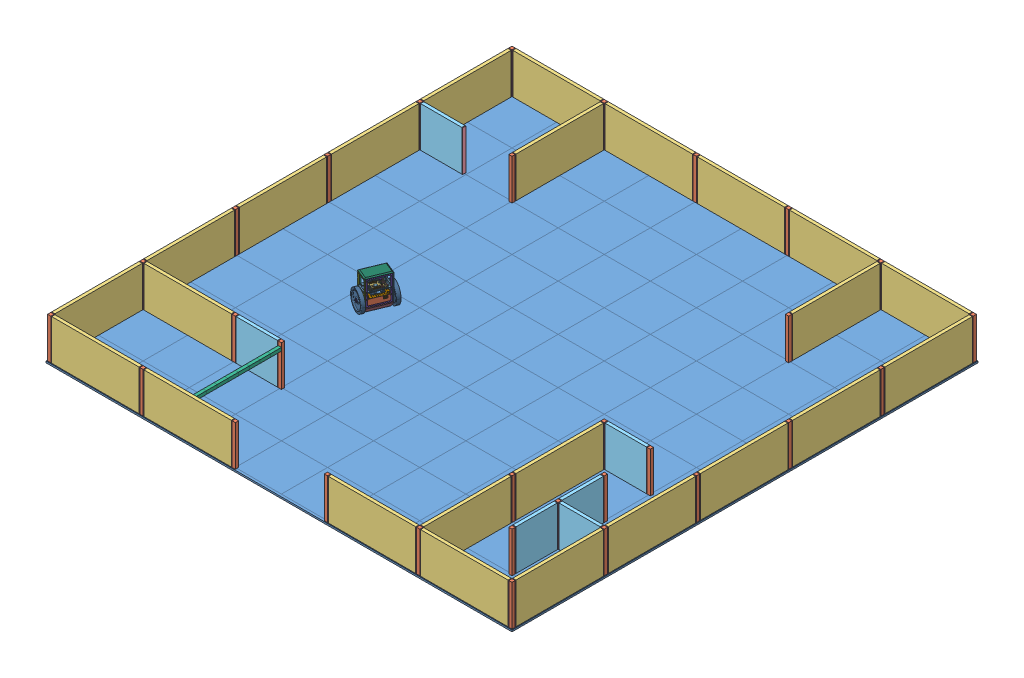
SolidWorks assembly testbed, configuration Default. Lengths in mm. (continued)
Components (placement in the parent): (continued)
- twipr-1: twipr [Default] at (-1820.3783 -75.269 -1556.7406) x (0.381849 0 -0.924225) z (0.924225 0 0.381849) size (189.01 198.92 123.83) (continued)
  - robot-hub-1: robot-hub [Default] at (-323.8774 211.7203 115.5) x (-1 0 0) z (0 1 0) size (91.46 70 13.31) (continued)
    - robot-hub.step-1: robot-hub.step [Default] at origin size (91.46 70 13.31) (continued)
      - Fuse_1206_3216Metric.step-1: Fuse_1206_3216Metric.step [Default] at (82.7 -138.7 -0.05) x (-1 0 0) z (0 0 -1) size (3.2 1.6 0.55)
        - SOLID-32.step-1: SOLID-32.step [Default] at origin size (3.2 1.6 0.55)
      - R_0603_1608Metric.step-24: R_0603_1608Metric.step [Default] at (125.4 -130.4 -0.05) x (0 -1 0) z (0 0 -1) size (1.6 0.8 0.45)
        - SOLID.step-1: SOLID.step [Default] at origin size (1.6 0.8 0.45)
      - R_0603_1608Metric.step-25: R_0603_1608Metric.step [Default] at (144.7 -142.2 -0.05) x (1 0 0) z (0 0 -1) size (1.6 0.8 0.45)
        - SOLID.step-1: SOLID.step [Default] at origin size (1.6 0.8 0.45)
      - R_0603_1608Metric.step-26: R_0603_1608Metric.step [Default] at (151.2 -84.3 -0.05) x (0 1 0) z (0 0 -1) size (1.6 0.8 0.45)
        - SOLID.step-1: SOLID.step [Default] at origin size (1.6 0.8 0.45)
      - R_0603_1608Metric.step-27: R_0603_1608Metric.step [Default] at (96 -137.2 -0.05) x (0 1 0) z (0 0 -1) size (1.6 0.8 0.45)
        - SOLID.step-1: SOLID.step [Default] at origin size (1.6 0.8 0.45)
      - R_0603_1608Metric.step-28: R_0603_1608Metric.step [Default] at (104.5 -106.1 -0.05) x (-1 0 0) z (0 0 -1) size (1.6 0.8 0.45)
        - SOLID.step-1: SOLID.step [Default] at origin size (1.6 0.8 0.45)
      - DF40C-100DS.step-1: DF40C-100DS.step [Default] at (144.62 -86.64 -0.05) x (0 -1 0) z (1 0 0) size (3.38 1.45 22.6)
        - SOLID-33.step-1: SOLID-33.step [Default] at origin size (3.38 1.45 22.6)
      - DF40C-100DS.step-2: DF40C-100DS.step [Default] at (144.62 -120.56 -0.05) x (0 -1 0) z (1 0 0) size (3.38 1.45 22.6)
        - SOLID-33.step-1: SOLID-33.step [Default] at origin size (3.38 1.45 22.6)
      - R_0603_1608Metric.step-29: R_0603_1608Metric.step [Default] at (96.8 -143.9 -0.05) x (0 -1 0) z (0 0 -1) size (1.6 0.8 0.45)
        - SOLID.step-1: SOLID.step [Default] at origin size (1.6 0.8 0.45)
      - C_0603_1608Metric.step-19: C_0603_1608Metric.step [Default] at (137.4625 -133.3 -0.05) x (0 1 0) z (0 0 -1) size (1.6 0.8 0.8)
        - SOLID-1.step-1: SOLID-1.step [Default] at origin size (1.6 0.8 0.8)
      - R_0603_1608Metric.step-30: R_0603_1608Metric.step [Default] at (92.9 -93.2 -0.05) x (0 -1 0) z (0 0 -1) size (1.6 0.8 0.45)
        - SOLID.step-1: SOLID.step [Default] at origin size (1.6 0.8 0.45)
      - C_0805_2012Metric.step-5: C_0805_2012Metric.step [Default] at (101.6 -119.9 -0.05) x (0 -1 0) z (0 0 -1) size (2 1.25 1.25)
        - SOLID-11.step-1: SOLID-11.step [Default] at origin size (2 1.25 1.25)
      - MC74VHC1G14DTT1G.step-1: MC74VHC1G14DTT1G.step [Default] at (157.4 -110.9 -0.05) x (0 -1 0) z (0 0 -1) size (2.75 3 1.1)
        - COMPOUND-34.step-1: COMPOUND-34.step [Default] at origin size (2.75 3 1.1)
      - R_0603_1608Metric.step-31: R_0603_1608Metric.step [Default] at (158.3 -115 -0.05) x (0 1 0) z (0 0 -1) size (1.6 0.8 0.45)
        - SOLID.step-1: SOLID.step [Default] at origin size (1.6 0.8 0.45)
      - C_0603_1608Metric.step-20: C_0603_1608Metric.step [Default] at (88.4 -93.2 -0.05) x (0 -1 0) z (0 0 -1) size (1.6 0.8 0.8)
        - SOLID-1.step-1: SOLID-1.step [Default] at origin size (1.6 0.8 0.8)
      - 9774030151 (rev1).step-1: 9774030151 (rev1).step [Default] at (160 -87.1 -0.05) x (-1 0 0) z (0 0 -1) size (5.1 5.89 4.4)
        - SOLID-35.step-1: SOLID-35.step [Default] at origin size (5.1 5.89 4.4)
      - D_SOD-323F.step-1: D_SOD-323F.step [Default] at (96.1 -113.45 -0.05) x (-1 0 0) z (0 0 -1) size (2.5 1.25 0.73)
        - SOLID-36.step-1: SOLID-36.step [Default] at origin size (2.5 1.25 0.73)
      - SM04B-SRSS-TB_dark.step-1: SM04B-SRSS-TB_dark.step [Default] at (86.2 -81 0.2) x (1 0 0) z (0 1 0) size (6 2.96 4.95)
        - SOLID-37.step-1: SOLID-37.step [Default] at origin size (6 2.96 4.95)
      - 9774030151 (rev1).step-2: 9774030151 (rev1).step [Default] at (112 -120.1 -0.05) x (-1 0 0) z (0 0 -1) size (5.1 5.89 4.4)
        - SOLID-35.step-1: SOLID-35.step [Default] at origin size (5.1 5.89 4.4)
      - M24512-DFDW6TP.step-1: M24512-DFDW6TP.step [Default] at (121.95 -135.9 -0.05) x (1 0 0) z (0 0 -1) size (6.4 3 1.2)
        - COMPOUND-38.step-1: COMPOUND-38.step [Default] at origin size (6.4 3 1.2)
      - C_0603_1608Metric.step-21: C_0603_1608Metric.step [Default] at (126.8 -141.9 -0.05) x (0 1 0) z (0 0 -1) size (1.6 0.8 0.8)
        - SOLID-1.step-1: SOLID-1.step [Default] at origin size (1.6 0.8 0.8)
      - IRF7319TRPBF.step-1: IRF7319TRPBF.step [Default] at (152.8 -137.5 -0.05) x (0 -1 0) z (0 0 -1) size (6 4.9 1.75)
        - COMPOUND-39.step-1: COMPOUND-39.step [Default] at origin size (6 4.9 1.75)
      - SX1508BIULTRT.step-1: SX1508BIULTRT.step [Default] at (120.1 -86 -0.05) x (-1 0 0) z (0 0 -1) size (3.1 3.1 0.6)
        - COMPOUND-40.step-1: COMPOUND-40.step [Default] at origin size (3.1 3.1 0.6)
      - R_0603_1608Metric.step-32: R_0603_1608Metric.step [Default] at (147.2 -130.6 -0.05) x (0 1 0) z (0 0 -1) size (1.6 0.8 0.45)
        - SOLID.step-1: SOLID.step [Default] at origin size (1.6 0.8 0.45)
      - LTC4365CTS8#TRMPBF.step-1: LTC4365CTS8#TRMPBF.step [Default] at (91.3 -135.6 -0.05) x (-1 0 0) z (0 0 -1) size (2.8 2.9 1)
        - COMPOUND-41.step-1: COMPOUND-41.step [Default] at origin size (2.8 2.9 1)
      - C_0603_1608Metric.step-22: C_0603_1608Metric.step [Default] at (106.5 -133.3 -0.05) x (0 -1 0) z (0 0 -1) size (1.6 0.8 0.8)
        - SOLID-1.step-1: SOLID-1.step [Default] at origin size (1.6 0.8 0.8)
      - SOT-323_SC-70.step-2: SOT-323_SC-70.step [Default] at (92.8 -112.95 -0.05) x (0 -1 0) z (0 0 -1) size (2 2 1.05)
        - SOLID-17.step-1: SOLID-17.step [Default] at origin size (2 2 1.05)
      - R_0603_1608Metric.step-33: R_0603_1608Metric.step [Default] at (112 -98.3 -0.05) x (0 1 0) z (0 0 -1) size (1.6 0.8 0.45)
        - SOLID.step-1: SOLID.step [Default] at origin size (1.6 0.8 0.45)
      - R_0603_1608Metric.step-34: R_0603_1608Metric.step [Default] at (149 -142.2 -0.05) x (-1 0 0) z (0 0 -1) size (1.6 0.8 0.45)
        - SOLID.step-1: SOLID.step [Default] at origin size (1.6 0.8 0.45)
      - R_0603_1608Metric.step-35: R_0603_1608Metric.step [Default] at (89.9 -139.3 -0.05) x (0 1 0) z (0 0 -1) size (1.6 0.8 0.45)
        - SOLID.step-1: SOLID.step [Default] at origin size (1.6 0.8 0.45)
      - R_0603_1608Metric.step-36: R_0603_1608Metric.step [Default] at (148.335 -134.9385 -0.05) x (0 1 0) z (0 0 -1) size (1.6 0.8 0.45)
        - SOLID.step-1: SOLID.step [Default] at origin size (1.6 0.8 0.45)
      - C_0805_2012Metric.step-6: C_0805_2012Metric.step [Default] at (99.5 -119.9 -0.05) x (0 -1 0) z (0 0 -1) size (2 1.25 1.25)
        - SOLID-11.step-1: SOLID-11.step [Default] at origin size (2 1.25 1.25)
      - C_0603_1608Metric.step-23: C_0603_1608Metric.step [Default] at (115.9 -144.25 -0.05) x (1 0 0) z (0 0 -1) size (1.6 0.8 0.8)
        - SOLID-1.step-1: SOLID-1.step [Default] at origin size (1.6 0.8 0.8)
      - LT3008ETS8#TRMPBF.step-1: LT3008ETS8#TRMPBF.step [Default] at (100.75 -135.5 -0.05) x (0 -1 0) z (0 0 -1) size (2.8 2.9 1)
        - COMPOUND-42.step-1: COMPOUND-42.step [Default] at origin size (2.8 2.9 1)
      - R_0603_1608Metric.step-37: R_0603_1608Metric.step [Default] at (132 -143.5 -0.05) x (0 -1 0) z (0 0 -1) size (1.6 0.8 0.45)
        - SOLID.step-1: SOLID.step [Default] at origin size (1.6 0.8 0.45)
      - R_0603_1608Metric.step-38: R_0603_1608Metric.step [Default] at (109.4 -107.2 -0.05) x (0 -1 0) z (0 0 -1) size (1.6 0.8 0.45)
        - SOLID.step-1: SOLID.step [Default] at origin size (1.6 0.8 0.45)
      - FM25V20A-DGQTR.step-1: FM25V20A-DGQTR.step [Default] at (129.9 -100.5 -0.05) x (-1 0 0) z (0 0 -1) size (6.1 5 0.8)
        - COMPOUND-43.step-1: COMPOUND-43.step [Default] at origin size (6.1 5 0.8)
      - R_0603_1608Metric.step-39: R_0603_1608Metric.step [Default] at (94.4 -135.4 -0.05) x (0 -1 0) z (0 0 -1) size (1.6 0.8 0.45)
        - SOLID.step-1: SOLID.step [Default] at origin size (1.6 0.8 0.45)
      - C_1210_3225Metric.step-7: C_1210_3225Metric.step [Default] at (104.4 -92 -0.05) x (-1 0 0) z (0 0 -1) size (3.2 2.5 2.5)
        - SOLID-0.step-1: SOLID-0.step [Default] at origin size (3.2 2.5 2.5)
      - SOT-323_SC-70.step-3: SOT-323_SC-70.step [Default] at (97 -134 -0.05) x (1 0 0) z (0 0 -1) size (2 2 1.05)
        - SOLID-17.step-1: SOLID-17.step [Default] at origin size (2 2 1.05)
      - SM04B-SRSS-TB_dark.step-2: SM04B-SRSS-TB_dark.step [Default] at (159.3 -135.7 0.2) x (0 -1 0) z (1 0 0) size (6 2.96 4.95)
        - SOLID-37.step-1: SOLID-37.step [Default] at origin size (6 2.96 4.95)
      - C_0603_1608Metric.step-24: C_0603_1608Metric.step [Default] at (116.8 -86.6 -0.05) x (0 -1 0) z (0 0 -1) size (1.6 0.8 0.8)
        - SOLID-1.step-1: SOLID-1.step [Default] at origin size (1.6 0.8 0.8)
      - C_0603_1608Metric.step-25: C_0603_1608Metric.step [Default] at (137.5 -140.9 -0.05) x (0 1 0) z (0 0 -1) size (1.6 0.8 0.8)
        - SOLID-1.step-1: SOLID-1.step [Default] at origin size (1.6 0.8 0.8)
      - C_0805_2012Metric.step-7: C_0805_2012Metric.step [Default] at (85.7 -87.2 -0.05) x (1 0 0) z (0 0 -1) size (2 1.25 1.25)
        - SOLID-11.step-1: SOLID-11.step [Default] at origin size (2 1.25 1.25)
      - IS25LP032D-JNLA3-TR.step-2: IS25LP032D-JNLA3-TR.step [Default] at (144.7 -137.5 -0.05) x (0 -1 0) z (0 0 -1) size (6 4.9 1.75)
        - COMPOUND-21.step-1: COMPOUND-21.step [Default] at origin size (6 4.9 1.75)
      - C_0603_1608Metric.step-26: C_0603_1608Metric.step [Default] at (128 -105.5 -0.05) x (0 1 0) z (0 0 -1) size (1.6 0.8 0.8)
        - SOLID-1.step-1: SOLID-1.step [Default] at origin size (1.6 0.8 0.8)
      - SOT-23-6.step-2: SOT-23-6.step [Default] at (102.8 -123.7 -0.05) x (-1 0 0) z (0 0 -1) size (2.8 2.9 1.55)
        - SOLID-24.step-1: SOLID-24.step [Default] at origin size (2.8 2.9 1.55)
      - PCT2075TP,147.step-1: PCT2075TP,147.step [Default] at (116 -141.3 -0.05) x (0 -1 0) z (0 0 -1) size (3.1 2 0.8)
        - COMPOUND-44.step-1: COMPOUND-44.step [Default] at origin size (3.1 2 0.8)
      - sk6812_side.step-1: sk6812_side.step [Default] at (75.35 -89.1 -1.05) x (0 -1 0) z (-1 0 0) size (4 2 1.6)
        - SOLID-45.step-1: SOLID-45.step [Default] at origin size (4 2 1.6)
      - R_0603_1608Metric.step-40: R_0603_1608Metric.step [Default] at (96 -111.5 -0.05) x (1 0 0) z (0 0 -1) size (1.6 0.8 0.45)
        - SOLID.step-1: SOLID.step [Default] at origin size (1.6 0.8 0.45)
      - R_0603_1608Metric.step-41: R_0603_1608Metric.step [Default] at (77.2 -90.65 -0.05) x (0 1 0) z (0 0 -1) size (1.6 0.8 0.45)
        - SOLID.step-1: SOLID.step [Default] at origin size (1.6 0.8 0.45)
      - C_0603_1608Metric.step-27: C_0603_1608Metric.step [Default] at (105.3 -137.6 -0.05) x (0 1 0) z (0 0 -1) size (1.6 0.8 0.8)
        - SOLID-1.step-1: SOLID-1.step [Default] at origin size (1.6 0.8 0.8)
      - STM32G031G6U6.step-2: STM32G031G6U6.step [Default] at (108.7 -137.5 -0.05) x (1 0 0) z (0 0 -1) size (4.1 4.1 0.6)
        - COMPOUND-31.step-1: COMPOUND-31.step [Default] at origin size (4.1 4.1 0.6)
      - SN74LVC3G17DCTR.step-1: SN74LVC3G17DCTR.step [Default] at (134.75 -142.2 -0.05) x (0 1 0) z (0 0 -1) size (4 2.95 1.3)
        - COMPOUND-46.step-1: COMPOUND-46.step [Default] at origin size (4 2.95 1.3)
      - R_0603_1608Metric.step-42: R_0603_1608Metric.step [Default] at (108.9 -109.7 -0.05) x (-1 0 0) z (0 0 -1) size (1.6 0.8 0.45)
        - SOLID.step-1: SOLID.step [Default] at origin size (1.6 0.8 0.45)
      - C_0805_2012Metric.step-8: C_0805_2012Metric.step [Default] at (94.8 -100.9 -0.05) x (0 1 0) z (0 0 -1) size (2 1.25 1.25)
        - SOLID-11.step-1: SOLID-11.step [Default] at origin size (2 1.25 1.25)
      - M24512-DFDW6TP.step-2: M24512-DFDW6TP.step [Default] at (121.95 -141.55 -0.05) x (1 0 0) z (0 0 -1) size (6.4 3 1.2)
        - COMPOUND-38.step-1: COMPOUND-38.step [Default] at origin size (6.4 3 1.2)
      - C_0603_1608Metric.step-28: C_0603_1608Metric.step [Default] at (101.6 -87.75 -0.05) x (1 0 0) z (0 0 -1) size (1.6 0.8 0.8)
        - SOLID-1.step-1: SOLID-1.step [Default] at origin size (1.6 0.8 0.8)
      - C_0603_1608Metric.step-29: C_0603_1608Metric.step [Default] at (108 -133.3 -0.05) x (0 -1 0) z (0 0 -1) size (1.6 0.8 0.8)
        - SOLID-1.step-1: SOLID-1.step [Default] at origin size (1.6 0.8 0.8)
      - R_0603_1608Metric.step-43: R_0603_1608Metric.step [Default] at (126.9 -130.4 -0.05) x (0 -1 0) z (0 0 -1) size (1.6 0.8 0.45)
        - SOLID.step-1: SOLID.step [Default] at origin size (1.6 0.8 0.45)
      - R_0603_1608Metric.step-44: R_0603_1608Metric.step [Default] at (141.135 -134.9385 -0.05) x (0 1 0) z (0 0 -1) size (1.6 0.8 0.45)
        - SOLID.step-1: SOLID.step [Default] at origin size (1.6 0.8 0.45)
      - SOT-23-6.step-3: SOT-23-6.step [Default] at (153.1 -91.8 -0.05) x (1 0 0) z (0 0 -1) size (2.8 2.9 1.55)
        - SOLID-24.step-1: SOLID-24.step [Default] at origin size (2.8 2.9 1.55)
      - R_0603_1608Metric.step-45: R_0603_1608Metric.step [Default] at (119.59 -119.2 -0.05) x (-1 0 0) z (0 0 -1) size (1.6 0.8 0.45)
        - SOLID.step-1: SOLID.step [Default] at origin size (1.6 0.8 0.45)
      - R_0603_1608Metric.step-46: R_0603_1608Metric.step [Default] at (128.5 -130.4 -0.05) x (0 -1 0) z (0 0 -1) size (1.6 0.8 0.45)
        - SOLID.step-1: SOLID.step [Default] at origin size (1.6 0.8 0.45)
      - R_0603_1608Metric.step-47: R_0603_1608Metric.step [Default] at (128.8 -109 -0.05) x (0 1 0) z (0 0 -1) size (1.6 0.8 0.45)
        - SOLID.step-1: SOLID.step [Default] at origin size (1.6 0.8 0.45)
      - C_0805_2012Metric.step-9: C_0805_2012Metric.step [Default] at (96.9 -100.9 -0.05) x (0 1 0) z (0 0 -1) size (2 1.25 1.25)
        - SOLID-11.step-1: SOLID-11.step [Default] at origin size (2 1.25 1.25)
      - R_0603_1608Metric.step-48: R_0603_1608Metric.step [Default] at (141.135 -138.0385 -0.05) x (0 -1 0) z (0 0 -1) size (1.6 0.8 0.45)
        - SOLID.step-1: SOLID.step [Default] at origin size (1.6 0.8 0.45)
      - SM04B-SRSS-TB_dark.step-3: SM04B-SRSS-TB_dark.step [Default] at (101.5 -142.1 0.2) x (-1 0 0) z (0 -1 0) size (6 2.96 4.95)
        - SOLID-37.step-1: SOLID-37.step [Default] at origin size (6 2.96 4.95)
      - C_0603_1608Metric.step-30: C_0603_1608Metric.step [Default] at (139.0125 -133.3 -0.05) x (0 1 0) z (0 0 -1) size (1.6 0.8 0.8)
        - SOLID-1.step-1: SOLID-1.step [Default] at origin size (1.6 0.8 0.8)
      - R_0603_1608Metric.step-49: R_0603_1608Metric.step [Default] at (152.7 -142.2 -0.05) x (1 0 0) z (0 0 -1) size (1.6 0.8 0.45)
        - SOLID.step-1: SOLID.step [Default] at origin size (1.6 0.8 0.45)
      - C_0805_2012Metric.step-10: C_0805_2012Metric.step [Default] at (85.75 -93.75 -0.05) x (1 0 0) z (0 0 -1) size (2 1.25 1.25)
        - SOLID-11.step-1: SOLID-11.step [Default] at origin size (2 1.25 1.25)
      - R_0603_1608Metric.step-50: R_0603_1608Metric.step [Default] at (127.7 -96.9 -0.05) x (1 0 0) z (0 0 -1) size (1.6 0.8 0.45)
        - SOLID.step-1: SOLID.step [Default] at origin size (1.6 0.8 0.45)
      - C_0805_2012Metric.step-11: C_0805_2012Metric.step [Default] at (100.75 -132.4 -0.05) x (1 0 0) z (0 0 -1) size (2 1.25 1.25)
        - SOLID-11.step-1: SOLID-11.step [Default] at origin size (2 1.25 1.25)
      - NCV8187AMLE330TCG.step-1: NCV8187AMLE330TCG.step [Default] at (96.2 -119.9 -0.05) x (-1 0 0) z (0 0 -1) size (3.1 3 1)
        - COMPOUND-47.step-1: COMPOUND-47.step [Default] at origin size (3.1 3 1)
      - R_0402_1005Metric.step-11: R_0402_1005Metric.step [Default] at (91.95 -87.35 -0.05) x (-1 0 0) z (0 0 -1) size (1 0.5 0.35)
        - SOLID-3.step-1: SOLID-3.step [Default] at origin size (1 0.5 0.35)
      - SOIC-16_3.9x9.9mm_P1.27mm.step-1: SOIC-16_3.9x9.9mm_P1.27mm.step [Default] at (96.9 -106.7 -0.05) x (0 1 0) z (0 0 -1) size (6 9.9 1.75)
        - SOLID-48.step-1: SOLID-48.step [Default] at origin size (6 9.9 1.75)
      - C_0603_1608Metric.step-31: C_0603_1608Metric.step [Default] at (96.8 -92.75 -0.05) x (-1 0 0) z (0 0 -1) size (1.6 0.8 0.8)
        - SOLID-1.step-1: SOLID-1.step [Default] at origin size (1.6 0.8 0.8)
      - R_0603_1608Metric.step-51: R_0603_1608Metric.step [Default] at (107.7 -107.2 -0.05) x (0 1 0) z (0 0 -1) size (1.6 0.8 0.45)
        - SOLID.step-1: SOLID.step [Default] at origin size (1.6 0.8 0.45)
      - R_0603_1608Metric.step-52: R_0603_1608Metric.step [Default] at (141.5 -130.7 -0.05) x (0 -1 0) z (0 0 -1) size (1.6 0.8 0.45)
        - SOLID.step-1: SOLID.step [Default] at origin size (1.6 0.8 0.45)
      - ECS-120-20-33-CKM-TR.step-1: ECS-120-20-33-CKM-TR.step [Default] at (104.7 -102.5 -0.05) x (0 1 0) z (0 0 -1) size (3.38 2.68 0.9)
        - COMPOUND-49.step-1: COMPOUND-49.step [Default] at origin size (3.38 2.68 0.9)
      - R_0603_1608Metric.step-53: R_0603_1608Metric.step [Default] at (93.5 -139.3 -0.05) x (0 -1 0) z (0 0 -1) size (1.6 0.8 0.45)
        - SOLID.step-1: SOLID.step [Default] at origin size (1.6 0.8 0.45)
      - C_0603_1608Metric.step-32: C_0603_1608Metric.step [Default] at (125.4 -99.5 -0.05) x (0 1 0) z (0 0 -1) size (1.6 0.8 0.8)
        - SOLID-1.step-1: SOLID-1.step [Default] at origin size (1.6 0.8 0.8)
      - R_0402_1005Metric.step-12: R_0402_1005Metric.step [Default] at (91.95 -88.35 -0.05) x (1 0 0) z (0 0 -1) size (1 0.5 0.35)
        - SOLID-3.step-1: SOLID-3.step [Default] at origin size (1 0.5 0.35)
      - 5033981892.step-1: 5033981892.step [Default] at (97.05 29.65 -154.55) x (0 -1 0) z (0 0 1) size (13.1 14.05 1.28)
        - COMPOUND-50.step-1: COMPOUND-50.step [Default] at origin size (13.1 14.05 1.28)
      - R_0603_1608Metric.step-54: R_0603_1608Metric.step [Default] at (131.9625 -136.35 -0.05) x (0 -1 0) z (0 0 -1) size (1.6 0.8 0.45)
        - SOLID.step-1: SOLID.step [Default] at origin size (1.6 0.8 0.45)
      - SOT-563.step-2: SOT-563.step [Default] at (89.5 -84.65 -0.05) x (-1 0 0) z (0 0 -1) size (1.6 1.6 0.63)
        - SOLID-29.step-1: SOLID-29.step [Default] at origin size (1.6 1.6 0.63)
      - R_0603_1608Metric.step-55: R_0603_1608Metric.step [Default] at (94.45 -93.2 -0.05) x (0 -1 0) z (0 0 -1) size (1.6 0.8 0.45)
        - SOLID.step-1: SOLID.step [Default] at origin size (1.6 0.8 0.45)
      - R_0603_1608Metric.step-56: R_0603_1608Metric.step [Default] at (123.9 -130.4 -0.05) x (0 -1 0) z (0 0 -1) size (1.6 0.8 0.45)
        - SOLID.step-1: SOLID.step [Default] at origin size (1.6 0.8 0.45)
      - R_0603_1608Metric.step-57: R_0603_1608Metric.step [Default] at (117 -100 -0.05) x (0 -1 0) z (0 0 -1) size (1.6 0.8 0.45)
        - SOLID.step-1: SOLID.step [Default] at origin size (1.6 0.8 0.45)
      - R_0603_1608Metric.step-58: R_0603_1608Metric.step [Default] at (91.7 -139.3 -0.05) x (0 -1 0) z (0 0 -1) size (1.6 0.8 0.45)
        - SOLID.step-1: SOLID.step [Default] at origin size (1.6 0.8 0.45)
      - R_0402_1005Metric.step-13: R_0402_1005Metric.step [Default] at (91.95 -89.35 -0.05) x (1 0 0) z (0 0 -1) size (1 0.5 0.35)
        - SOLID-3.step-1: SOLID-3.step [Default] at origin size (1 0.5 0.35)
      - sk6812_side.step-2: sk6812_side.step [Default] at (75.35 -96.1 -1.05) x (0 -1 0) z (-1 0 0) size (4 2 1.6)
        - SOLID-45.step-1: SOLID-45.step [Default] at origin size (4 2 1.6)
      - R_0603_1608Metric.step-59: R_0603_1608Metric.step [Default] at (118.6 -100 -0.05) x (0 -1 0) z (0 0 -1) size (1.6 0.8 0.45)
        - SOLID.step-1: SOLID.step [Default] at origin size (1.6 0.8 0.45)
      - C_0805_2012Metric.step-12: C_0805_2012Metric.step [Default] at (92.9 -119.9 -0.05) x (0 -1 0) z (0 0 -1) size (2 1.25 1.25)
        - SOLID-11.step-1: SOLID-11.step [Default] at origin size (2 1.25 1.25)
      - C_0805_2012Metric.step-13: C_0805_2012Metric.step [Default] at (103.5 -135.8 -0.05) x (0 1 0) z (0 0 -1) size (2 1.25 1.25)
        - SOLID-11.step-1: SOLID-11.step [Default] at origin size (2 1.25 1.25)
      - SM04B-SRSS-TB_dark.step-4: SM04B-SRSS-TB_dark.step [Default] at (159.3 -127.9 0.2) x (0 -1 0) z (1 0 0) size (6 2.96 4.95)
        - SOLID-37.step-1: SOLID-37.step [Default] at origin size (6 2.96 4.95)
      - C_0603_1608Metric.step-33: C_0603_1608Metric.step [Default] at (78.75 -90.65 -0.05) x (0 1 0) z (0 0 -1) size (1.6 0.8 0.8)
        - SOLID-1.step-1: SOLID-1.step [Default] at origin size (1.6 0.8 0.8)
      - SN74LVC3G17DCTR.step-2: SN74LVC3G17DCTR.step [Default] at (134.7125 -134.9 -0.05) x (0 1 0) z (0 0 -1) size (4 2.95 1.3)
        - COMPOUND-46.step-1: COMPOUND-46.step [Default] at origin size (4 2.95 1.3)
      - DMS0008A.step-1: DMS0008A.step [Default] at (85.1 -135.6 -0.05) x (-1 0 0) z (0 0 -1) size (3.3 3.3 0.8)
        - COMPOUND-51.step-1: COMPOUND-51.step [Default] at origin size (3.3 3.3 0.8)
      - TPS22975NDSGT.step-1: TPS22975NDSGT.step [Default] at (104.8 -88.5 -0.05) x (0 1 0) z (0 0 -1) size (2 2 0.78)
        - COMPOUND-52.step-1: COMPOUND-52.step [Default] at origin size (2 2 0.78)
      - R_0603_1608Metric.step-60: R_0603_1608Metric.step [Default] at (143.1 -130.7 -0.05) x (0 -1 0) z (0 0 -1) size (1.6 0.8 0.45)
        - SOLID.step-1: SOLID.step [Default] at origin size (1.6 0.8 0.45)
      - Fuse_1206_3216Metric.step-2: Fuse_1206_3216Metric.step [Default] at (107.4 -86.4 -0.05) x (0 1 0) z (0 0 -1) size (3.2 1.6 0.55)
        - SOLID-32.step-1: SOLID-32.step [Default] at origin size (3.2 1.6 0.55)
      - SM04B-SRSS-TB_dark.step-5: SM04B-SRSS-TB_dark.step [Default] at (94 -81 0.2) x (1 0 0) z (0 1 0) size (6 2.96 4.95)
        - SOLID-37.step-1: SOLID-37.step [Default] at origin size (6 2.96 4.95)
      - R_0603_1608Metric.step-61: R_0603_1608Metric.step [Default] at (115.7 -89.4 -0.05) x (-1 0 0) z (0 0 -1) size (1.6 0.8 0.45)
        - SOLID.step-1: SOLID.step [Default] at origin size (1.6 0.8 0.45)
      - R_0603_1608Metric.step-62: R_0603_1608Metric.step [Default] at (101.2 -129.6 -0.05) x (0 -1 0) z (0 0 -1) size (1.6 0.8 0.45)
        - SOLID.step-1: SOLID.step [Default] at origin size (1.6 0.8 0.45)
      - R_0603_1608Metric.step-63: R_0603_1608Metric.step [Default] at (148.335 -138.0385 -0.05) x (0 1 0) z (0 0 -1) size (1.6 0.8 0.45)
        - SOLID.step-1: SOLID.step [Default] at origin size (1.6 0.8 0.45)
      - PCT2075TP,147.step-2: PCT2075TP,147.step [Default] at (125 -105.6 -0.05) x (1 0 0) z (0 0 -1) size (3.1 2 0.8)
        - COMPOUND-44.step-1: COMPOUND-44.step [Default] at origin size (3.1 2 0.8)
      - R_0603_1608Metric.step-64: R_0603_1608Metric.step [Default] at (101.6 -89.35 -0.05) x (1 0 0) z (0 0 -1) size (1.6 0.8 0.45)
        - SOLID.step-1: SOLID.step [Default] at origin size (1.6 0.8 0.45)
      - R_0603_1608Metric.step-65: R_0603_1608Metric.step [Default] at (149.6 -109.1 -0.05) x (0 -1 0) z (0 0 -1) size (1.6 0.8 0.45)
        - SOLID.step-1: SOLID.step [Default] at origin size (1.6 0.8 0.45)
      - R_0603_1608Metric.step-66: R_0603_1608Metric.step [Default] at (153 -84.3 -0.05) x (0 1 0) z (0 0 -1) size (1.6 0.8 0.45)
        - SOLID.step-1: SOLID.step [Default] at origin size (1.6 0.8 0.45)
      - C_0603_1608Metric.step-34: C_0603_1608Metric.step [Default] at (132 -140.4 -0.05) x (0 1 0) z (0 0 -1) size (1.6 0.8 0.8)
        - SOLID-1.step-1: SOLID-1.step [Default] at origin size (1.6 0.8 0.8)
      - C_0603_1608Metric.step-35: C_0603_1608Metric.step [Default] at (151.45 -132.75 -0.05) x (-1 0 0) z (0 0 -1) size (1.6 0.8 0.8)
        - SOLID-1.step-1: SOLID-1.step [Default] at origin size (1.6 0.8 0.8)
      - R_0603_1608Metric.step-67: R_0603_1608Metric.step [Default] at (101.4 -101.2 -0.05) x (0 1 0) z (0 0 -1) size (1.6 0.8 0.45)
        - SOLID.step-1: SOLID.step [Default] at origin size (1.6 0.8 0.45)
      - R_0603_1608Metric.step-68: R_0603_1608Metric.step [Default] at (108.9 -111.2 -0.05) x (-1 0 0) z (0 0 -1) size (1.6 0.8 0.45)
        - SOLID.step-1: SOLID.step [Default] at origin size (1.6 0.8 0.45)
      - Fuse_1206_3216Metric.step-3: Fuse_1206_3216Metric.step [Default] at (90.5 -120.5 -0.05) x (0 -1 0) z (0 0 -1) size (3.2 1.6 0.55)
        - SOLID-32.step-1: SOLID-32.step [Default] at origin size (3.2 1.6 0.55)
      - robot-hub_rev3 PCB.step-1: robot-hub_rev3 PCB.step [Default] at origin size (90 70 1.66)
  - bat_compartment-1: bat_compartment [Default] at (-442.6774 127.2203 0) x (-1 0 0) z (0 0 1) size (140 30 80)
  - platform_control-1: platform_control [Default] at (-442.6774 200.7203 -0.1) size (140 11 78)
  - marker_top-1: marker_top [Default] at (-442.6774 277.2203 0) size (140 14 80)
  - socket head cap screw_din-2: socket head cap screw_din [DIN 912 M2.5 x 4 --- 4N] at (-375.1774 237.7203 -36.5) x (-1 0 0) z (0 0.924225 0.381849) size (6.5 4.5 4.5)
  - socket head cap screw_din-3: socket head cap screw_din [DIN 912 M2.5 x 4 --- 4N] at (-375.1774 237.7203 36.5) x (-1 0 0) z (0 0.924225 0.381849) size (6.5 4.5 4.5)
  - socket head cap screw_din-4: socket head cap screw_din [DIN 912 M2.5 x 4 --- 4N] at (-375.1774 273.7203 36.5) x (-1 0 0) z (0 0.924225 0.381849) size (6.5 4.5 4.5)
  - socket head cap screw_din-5: socket head cap screw_din [DIN 912 M2.5 x 4 --- 4N] at (-375.1774 273.7203 -36.5) x (-1 0 0) z (0 0.924225 0.381849) size (6.5 4.5 4.5)
  - socket head cap screw_din-6: socket head cap screw_din [DIN 912 M2.5 x 4 --- 4N] at (-383.1774 204.2203 -39.5) x (0 0 1) z (-1 0 0) size (6.5 4.5 4.5)
  - socket head cap screw_din-7: socket head cap screw_din [DIN 912 M2.5 x 4 --- 4N] at (-502.1774 204.2203 -39.5) x (0 0 1) z (-1 0 0) size (6.5 4.5 4.5)
  - socket head cap screw_din-8: socket head cap screw_din [DIN 912 M2.5 x 4 --- 4N] at (-402.6774 133.7203 -36.5) x (0 -1 0) z (0 0 1) size (6.5 4.5 4.5)
  - socket head cap screw_din-9: socket head cap screw_din [DIN 912 M2.5 x 4 --- 4N] at (-482.6774 133.7203 -36.5) x (0 -1 0) z (0 0 1) size (6.5 4.5 4.5)
  - socket head cap screw_din-10: socket head cap screw_din [DIN 912 M2.5 x 4 --- 4N] at (-401.6774 215.8803 -27.1) x (0 -1 0) z (0 0 1) size (6.5 4.5 4.5)
  - socket head cap screw_din-11: socket head cap screw_din [DIN 912 M2.5 x 4 --- 4N] at (-483.6774 215.8803 -27.1) x (0 -1 0) z (0 0 1) size (6.5 4.5 4.5)
  - socket head cap screw_din-12: socket head cap screw_din [DIN 912 M2.5 x 4 --- 4N] at (-510.1774 237.7203 -36.5) size (6.5 4.5 4.5)
  - socket head cap screw_din-13: socket head cap screw_din [DIN 912 M2.5 x 4 --- 4N] at (-510.1774 273.7203 -36.5) size (6.5 4.5 4.5)
  - socket head cap screw_din-14: socket head cap screw_din [DIN 912 M2.5 x 4 --- 4N] at (-510.1774 273.7203 36.5) size (6.5 4.5 4.5)
  - socket head cap screw_din-15: socket head cap screw_din [DIN 912 M2.5 x 4 --- 4N] at (-510.1774 237.7203 36.5) size (6.5 4.5 4.5)
  - socket head cap screw_din-16: socket head cap screw_din [DIN 912 M2.5 x 4 --- 4N] at (-483.6774 215.8803 34.9) x (0 -1 0) z (0 0 1) size (6.5 4.5 4.5)
  - socket head cap screw_din-17: socket head cap screw_din [DIN 912 M2.5 x 4 --- 4N] at (-401.6774 215.8803 34.9) x (0 -1 0) z (0 0 1) size (6.5 4.5 4.5)
  - socket head cap screw_din-18: socket head cap screw_din [DIN 912 M2.5 x 4 --- 4N] at (-482.6774 133.7203 36.5) x (0 -1 0) z (0 0 1) size (6.5 4.5 4.5)
  - socket head cap screw_din-19: socket head cap screw_din [DIN 912 M2.5 x 4 --- 4N] at (-402.6774 133.7203 36.5) x (0 -1 0) z (0 0 1) size (6.5 4.5 4.5)
  - socket head cap screw_din-20: socket head cap screw_din [DIN 912 M2.5 x 4 --- 4N] at (-375.1774 175.7203 -36.5) x (-1 0 0) z (0 0.924225 0.381849) size (6.5 4.5 4.5)
  - socket head cap screw_din-21: socket head cap screw_din [DIN 912 M2.5 x 4 --- 4N] at (-375.1774 130.7203 -36.5) x (-1 0 0) z (0 0.924225 0.381849) size (6.5 4.5 4.5)
  - socket head cap screw_din-22: socket head cap screw_din [DIN 912 M2.5 x 4 --- 4N] at (-375.1774 130.7203 36.5) x (-1 0 0) z (0 0.924225 0.381849) size (6.5 4.5 4.5)
  - socket head cap screw_din-23: socket head cap screw_din [DIN 912 M2.5 x 4 --- 4N] at (-375.1774 175.7203 36.5) x (-1 0 0) z (0 0.924225 0.381849) size (6.5 4.5 4.5)
  - socket head cap screw_din-24: socket head cap screw_din [DIN 912 M2.5 x 4 --- 4N] at (-510.1774 130.7203 -36.5) size (6.5 4.5 4.5)
  - socket head cap screw_din-25: socket head cap screw_din [DIN 912 M2.5 x 4 --- 4N] at (-510.1774 175.7203 -36.5) size (6.5 4.5 4.5)
  - socket head cap screw_din-26: socket head cap screw_din [DIN 912 M2.5 x 4 --- 4N] at (-510.1774 175.7203 36.5) size (6.5 4.5 4.5)
  - socket head cap screw_din-27: socket head cap screw_din [DIN 912 M2.5 x 4 --- 4N] at (-510.1774 130.7203 36.5) size (6.5 4.5 4.5)
  - socket head cap screw_din-28: socket head cap screw_din [DIN 912 M3 x 5 --- 5N] at (-512.6774 160.2203 13) size (8 5.5 5.5)
  - socket head cap screw_din-29: socket head cap screw_din [DIN 912 M3 x 5 --- 5N] at (-512.6774 160.2203 -13) size (8 5.5 5.5)
  - socket head cap screw_din-30: socket head cap screw_din [DIN 912 M3 x 5 --- 5N] at (-512.6774 134.2203 -13) size (8 5.5 5.5)
  - socket head cap screw_din-31: socket head cap screw_din [DIN 912 M3 x 5 --- 5N] at (-512.6774 134.2203 13) size (8 5.5 5.5)
  - socket head cap screw_din-32: socket head cap screw_din [DIN 912 M3 x 5 --- 5N] at (-372.6774 134.2203 13) x (-1 0 0) z (0 0.924225 0.381849) size (8 5.5 5.5)
  - socket head cap screw_din-33: socket head cap screw_din [DIN 912 M3 x 5 --- 5N] at (-372.6774 160.2203 13) x (-1 0 0) z (0 0.924225 0.381849) size (8 5.5 5.5)
  - socket head cap screw_din-34: socket head cap screw_din [DIN 912 M3 x 5 --- 5N] at (-372.6774 160.2203 -13) x (-1 0 0) z (0 0.924225 0.381849) size (8 5.5 5.5)
  - socket head cap screw_din-35: socket head cap screw_din [DIN 912 M3 x 5 --- 5N] at (-372.6774 134.2203 -13) x (-1 0 0) z (0 0.924225 0.381849) size (8 5.5 5.5)
  - socket head cap screw_din-36: socket head cap screw_din [DIN 912 M2.5 x 4 --- 4N] at (-502.1774 166.7203 39.5) x (0 0 -1) z (1 0 0) size (6.5 4.5 4.5)
  - socket head cap screw_din-37: socket head cap screw_din [DIN 912 M2.5 x 4 --- 4N] at (-383.1774 166.7203 39.5) x (0 0 -1) z (1 0 0) size (6.5 4.5 4.5)
  - socket head cap screw_din-38: socket head cap screw_din [DIN 912 M2.5 x 4 --- 4N] at (-383.1774 204.2203 39.5) x (0 0 -1) z (1 0 0) size (6.5 4.5 4.5)
  - socket head cap screw_din-39: socket head cap screw_din [DIN 912 M2.5 x 4 --- 4N] at (-502.1774 204.2203 39.5) x (0 0 -1) z (1 0 0) size (6.5 4.5 4.5)
  - socket head cap screw_din-40: socket head cap screw_din [DIN 912 M2.5 x 4 --- 4N] at (-383.1774 166.2203 -39.5) x (0 0 1) z (-1 0 0) size (6.5 4.5 4.5)
  - socket head cap screw_din-41: socket head cap screw_din [DIN 912 M2.5 x 4 --- 4N] at (-502.1774 166.2203 -39.5) x (0 0 1) z (-1 0 0) size (6.5 4.5 4.5)
  - T81H-RM41.stp-1: T81H-RM41.stp [Default] at (-368.6774 147.2203 0) x (0 0 -1) z (1 0 0) size (20.32 20.32 20.32)
  - T81H-RM41.stp-2: T81H-RM41.stp [Default] at (-516.6774 147.2203 0) x (0 0 1) z (-1 0 0) size (20.32 20.32 20.32)
  - bat_compartment_lid-1: bat_compartment_lid [Default] at (-442.6774 127.2203 0) x (-1 0 0) z (0 0 1) size (125.4 4 62)
  - SimpleBMS-1: SimpleBMS [Default] at (-264.9746 172.7203 56) x (-1 0 0) z (0 1 0) size (70 50 11.7)
  - cover_1-1: cover_1 [Default] at (-442.6774 151.9703 40) x (-1 0 0) z (0 0 -1) size (111.2 35.5 3)
  - cover_2-1: cover_2 [Default] at (-442.6774 151.9703 -40) size (111.2 35.5 3)
  - SE020A_01a-1: SE020A_01a [Default] at (-382.6774 147.2203 0) x (0 1 0) z (0 0 1) size (35.71 70 44.21)
  - SE020A_01a-2: SE020A_01a [Default] at (-502.6774 147.2203 0) x (0 -1 0) z (0 0 1) size (35.71 70 44.21)
- wallelement_1-cell-1: wallelement_1-cell [Default] at (-152.5 135 -285) x (0 0 -1) z (1 0 0) size (265 250 20)
  - wall_1-cell-1: wall_1-cell [Default] at origin size (255 250 20)
  - wall_profile_hook_250-1: wall_profile_hook_250 [Default] at (132.5 0 10) x (0 0 1) z (-1 0 0) size (20 250 5)
  - wall_profile_hook_250-2: wall_profile_hook_250 [Default] at (-132.5 0 10) x (0 0 -1) z (1 0 0) size (20 250 5)
- wallelement_1-cell-2: wallelement_1-cell [Default] at (-152.5 135 -570) x (0 0 -1) z (1 0 0) size (265 250 20)
  - wall_1-cell-1: wall_1-cell [Default] at origin size (255 250 20)
  - wall_profile_hook_250-1: wall_profile_hook_250 [Default] at (132.5 0 10) x (0 0 1) z (-1 0 0) size (20 250 5)
  - wall_profile_hook_250-2: wall_profile_hook_250 [Default] at (-132.5 0 10) x (0 0 -1) z (1 0 0) size (20 250 5)
- wallelement_1-cell-3: wallelement_1-cell [Default] at (0 135 -437.5) size (265 250 20)
  - wall_1-cell-1: wall_1-cell [Default] at origin size (255 250 20)
  - wall_profile_hook_250-1: wall_profile_hook_250 [Default] at (132.5 0 10) x (0 0 1) z (-1 0 0) size (20 250 5)
  - wall_profile_hook_250-2: wall_profile_hook_250 [Default] at (-132.5 0 10) x (0 0 -1) z (1 0 0) size (20 250 5)
- wallelement_1-cell-4: wallelement_1-cell [Default] at (-285 135 -1007.5) size (265 250 20)
  - wall_1-cell-1: wall_1-cell [Default] at origin size (255 250 20)
  - wall_profile_hook_250-1: wall_profile_hook_250 [Default] at (132.5 0 10) x (0 0 1) z (-1 0 0) size (20 250 5)
  - wall_profile_hook_250-2: wall_profile_hook_250 [Default] at (-132.5 0 10) x (0 0 -1) z (1 0 0) size (20 250 5)
